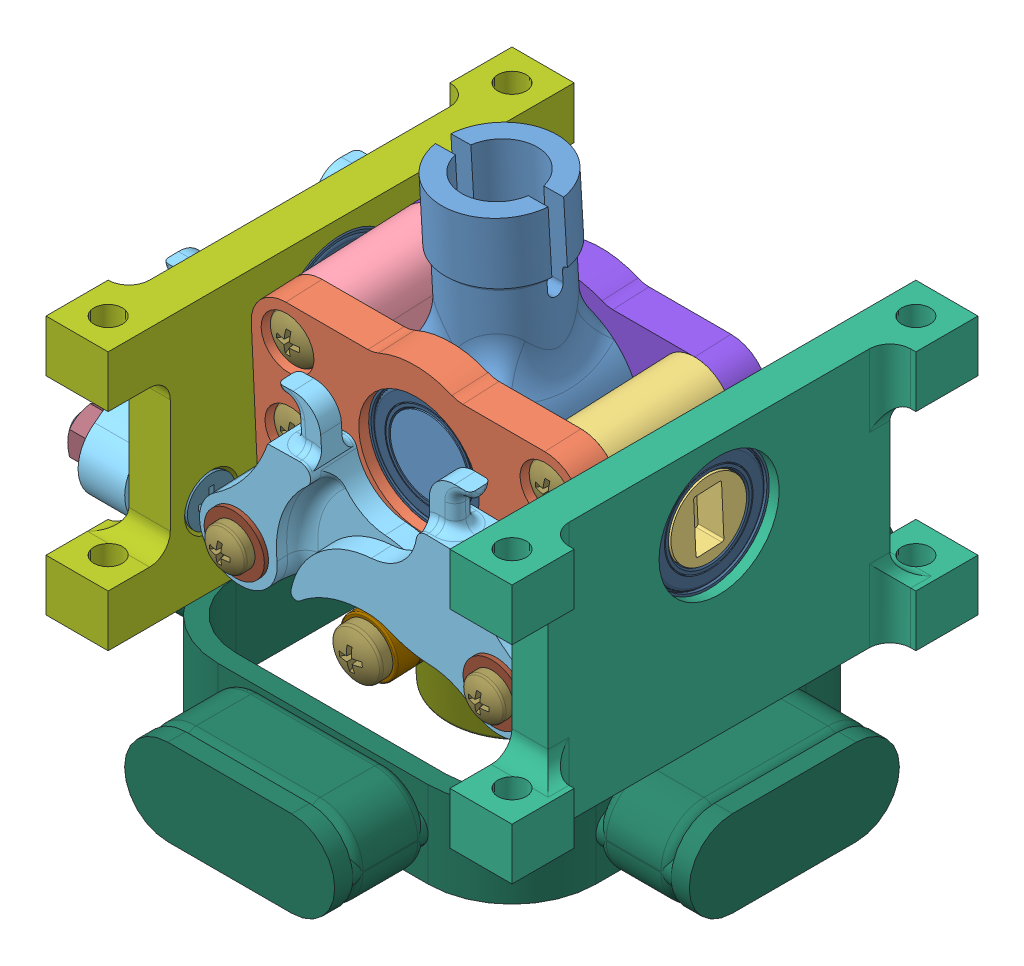
SolidWorks assembly gimbal, configuration Default. Lengths in mm.
Overall size (112.58 92.62 109.06).
47 component instances, 16 part files, 116 mates.
Components (placement in the parent):
- gimbal_lever_arm-1: gimbal_lever_arm [Default] at (47.4383 75.9682 -14.122) x (-0.999902 -0.01398 -0.000647) z (0 -0.046209 0.998932) size (30 86 35)
- gimbal_core_bearing_carrier_non_pot_side-1: gimbal_core_bearing_carrier_non_pot_side [Default] at (1 7.5205 9.7406) x (1 0 0) z (0 -0.046209 0.998932) size (64 44 7.5)
- gimbal_core_pot_side-1: gimbal_core_pot_side [Default] at (51 19.5077 10.2951) x (0 0.046209 -0.998932) z (1 0 0) size (22 30 20)
- gimbal_core_non_pot_side-1: gimbal_core_non_pot_side [Default] at (15 3.5756 -13.1836) x (0 -0.046209 0.998932) z (-1 0 0) size (23.38 47 23)
- gimbal_cam-1: gimbal_cam [Default] at (65.2863 3.5447 27.3757) x (-0.999775 0.021174 0.000979) z (0 0.046209 -0.998932) size (47.46 36.5 9)
- gimbal_cam-2: gimbal_cam [Default] at (0.7009 3.9697 18.3858) x (0.999801 0.01992 0.000921) z (0 -0.046209 0.998932) size (47.46 36.5 9)
- gimbal_frame_pot_side-1: gimbal_frame_pot_side [Default] at (66 0 45) x (0 0 -1) z (1 0 0) size (90 50 12)
- gimbal_frame_cam_side-1: gimbal_frame_cam_side [Default] at (0 0 -45) x (0 0 1) z (-1 0 0) size (90 50 12)
- gimbal_cam-3: gimbal_cam [Default] at (-18.3 4.8402 32.2821) x (0 0.021614 -0.999766) z (1 0 0) size (47.46 36.5 9)
- gimbal_cam-4: gimbal_cam [Default] at (-9.3 4.7894 -32.2106) x (0 0.028628 0.99959) z (-1 0 0) size (47.46 36.5 9)
- gimbal_core_bearing_carrier_pot_side-1: gimbal_core_bearing_carrier_pot_side [Default] at (65 18.027 -11.7969) x (-1 0 0) z (0 0.046209 -0.998932) size (64 34.5 7)
- 685 Bearing-1: 685 Bearing [По умолчанию] at (31.1601 10.3423 18.18) x (0 -0.046209 0.998932) z (-0.482505 -0.874958 -0.040474) size (5 11 11)
- 6802 Bearing-1: 6802 Bearing [Default] at (-2.5 35 0) x (1 0 0) z (0 -0.265463 0.964121) size (5 24 24)
- 6802 Bearing-2: 6802 Bearing [Default] at (68.5 35 0) x (1 0 0) z (0 -0.094888 0.995488) size (5 24 24)
- 6802 Bearing-3: 6802 Bearing [Default] at (33 34.3762 13.4856) x (0 0.046209 -0.998932) z (0.974697 -0.223291 -0.010329) size (5 24 24)
- 6802 Bearing-4: 6802 Bearing [Default] at (33 35.6238 -13.4856) x (0 -0.046209 0.998932) z (-0.998311 -0.058031 -0.002684) size (5 24 24)
- 685 Bearing-3: 685 Bearing [По умолчанию] at (-8.8 11.9085 -2.8011) x (-1 0 0) z (0 -0.658338 -0.752723) size (5 11 11)
- 685 Bearing-5: 685 Bearing [По умолчанию] at (-18.8 12.2864 -0.0857) x (1 0 0) z (0 -0.427815 0.903866) size (5 11 11)
- 685 Bearing-6: 685 Bearing [По умолчанию] at (33.1012 11.3912 23.2339) x (0 -0.046209 0.998932) z (-0.995039 -0.09938 -0.004597) size (5 11 11)
- MF105 Bearing-1: MF105 Bearing [Default] at (58 13.746 26.6463) x (-0.997509 0.070457 0.003259) z (0 0.046209 -0.998932) size (11.6 11.6 4)
- MF105 Bearing-2: MF105 Bearing [Default] at (58 14.051 20.0534) x (1 0 0) z (0 -0.046209 0.998932) size (11.6 11.6 4)
- MF105 Bearing-3: MF105 Bearing [Default] at (8 14.051 20.0534) x (1 0 0) z (0 -0.046209 0.998932) size (11.6 11.6 4)
- MF105 Bearing-4: MF105 Bearing [Default] at (8 13.746 26.6463) x (-0.996576 0.082596 0.003821) z (0 0.046209 -0.998932) size (11.6 11.6 4)
- MF105 Bearing-5: MF105 Bearing [Default] at (-10.5 15 25) x (0 0 1) z (-1 0 0) size (11.6 11.6 4)
- MF105 Bearing-6: MF105 Bearing [Default] at (-17.1 15 25) x (0 0.244393 -0.969676) z (1 0 0) size (11.6 11.6 4)
- MF105 Bearing-7: MF105 Bearing [Default] at (-17.1 15 -25) x (0 0 -1) z (1 0 0) size (11.6 11.6 4)
- MF105 Bearing-8: MF105 Bearing [Default] at (-10.5 15 -25) x (0 0 1) z (-1 0 0) size (11.6 11.6 4)
- pan cross head_am-1: pan cross head_am [B18.6.7M - M5 x 0.8 x 30 Type I Cross Recessed PHMS --30N] at (33.3499 8.5043 31.8096) x (0 0.046209 -0.998932) z (0.071714 -0.99636 -0.04609) size (33.67 9.5 9.5)
- pan cross head_am-2: pan cross head_am [B18.6.7M - M5 x 0.8 x 30 Type I Cross Recessed PHMS --30N] at (-22.5 10.0267 -1.1552) x (1 0 0) z (0 0.654485 0.756075) size (33.67 9.5 9.5)
- pan cross head_am-4: pan cross head_am [B18.6.7M - M4 x 0.7 x 20 Type I Cross Recessed PHMS --20N] at (8 13.5103 31.7409) x (0 0.046209 -0.998932) z (0.997483 -0.070827 -0.003276) size (23.07 8 8)
- pan cross head_am-5: pan cross head_am [B18.6.7M - M4 x 0.7 x 20 Type I Cross Recessed PHMS --20N] at (58 13.5103 31.7409) x (0 0.046209 -0.998932) z (0.997483 -0.070827 -0.003276) size (23.07 8 8)
- pan cross head_am-8: pan cross head_am [B18.6.7M - M5 x 0.8 x 35 Type I Cross Recessed PHMS --35N] at (58 42.1505 18.5502) x (0 0.046209 -0.998932) z (0.997483 -0.070827 -0.003276) size (38.67 9.5 9.5)
- pan cross head_am-9: pan cross head_am [B18.6.7M - M5 x 0.8 x 35 Type I Cross Recessed PHMS --35N] at (8 42.1505 18.5502) x (0 0.046209 -0.998932) z (0.997483 -0.070827 -0.003276) size (38.67 9.5 9.5)
- pan cross head_am-10: pan cross head_am [B18.6.7M - M5 x 0.8 x 35 Type I Cross Recessed PHMS --35N] at (8 26.1675 17.8109) x (0 0.046209 -0.998932) z (0.997483 -0.070827 -0.003276) size (38.67 9.5 9.5)
- pan cross head_am-11: pan cross head_am [B18.6.7M - M5 x 0.8 x 35 Type I Cross Recessed PHMS --35N] at (58 26.1675 17.8109) x (0 0.046209 -0.998932) z (0.997483 -0.070827 -0.003276) size (38.67 9.5 9.5)
- hex nut style 1_am-1: hex nut style 1_am [B18.2.4.1M - Hex nut, Style 1,  M5 x 0.8 --D-N] at (8 43.8787 -18.8098) x (0.866025 0.499466 0.023104) z (0 0.046209 -0.998932) size (8 9.24 4.7)
- hex nut style 1_am-2: hex nut style 1_am [B18.2.4.1M - Hex nut, Style 1,  M5 x 0.8 --D-N] at (8 27.8958 -19.5492) x (0.866025 0.499466 0.023104) z (0 0.046209 -0.998932) size (8 9.24 4.7)
- hex nut style 1_am-3: hex nut style 1_am [B18.2.4.1M - Hex nut, Style 1,  M5 x 0.8 --D-N] at (58 27.8958 -19.5492) x (0.866025 -0.499466 -0.023104) z (0 0.046209 -0.998932) size (8 9.24 4.7)
- hex nut style 1_am-4: hex nut style 1_am [B18.2.4.1M - Hex nut, Style 1,  M5 x 0.8 --D-N] at (58 43.8787 -18.8098) x (0.866025 -0.499466 -0.023104) z (0 0.046209 -0.998932) size (8 9.24 4.7)
- flat head screw_am-1: flat head screw_am [B18.6.7M - M5 x 0.8 x 25 Type I Cross Recessed FHMS --25N] at (-0.05 15 -25) x (-1 0 0) z (0 -0.000444 -1) size (25 9.3 9.3)
- flat head screw_am-2: flat head screw_am [B18.6.7M - M5 x 0.8 x 25 Type I Cross Recessed FHMS --25N] at (-0.05 15 25) x (-1 0 0) z (0 -0.006616 -0.999978) size (25 9.3 9.3)
- hex nut style 1_am-5: hex nut style 1_am [B18.2.4.1M - Hex nut, Style 1,  M5 x 0.8 --D-N] at (-23.8 15 25) x (0 0 1) z (-1 0 0) size (8 9.24 4.7)
- hex nut style 1_am-6: hex nut style 1_am [B18.2.4.1M - Hex nut, Style 1,  M5 x 0.8 --D-N] at (-23.8 15 -25) x (0 0 1) z (-1 0 0) size (8 9.24 4.7)
- hex nut style 1_am-9: hex nut style 1_am [B18.2.4.1M - Hex nut, Style 1,  M5 x 0.8 --D-N] at (58 14.5685 8.8654) x (0.866025 0.499466 0.023104) z (0 0.046209 -0.998932) size (8 9.24 4.7)
- hex nut style 1_am-10: hex nut style 1_am [B18.2.4.1M - Hex nut, Style 1,  M5 x 0.8 --D-N] at (8 14.5685 8.8654) x (0.866025 -0.499466 -0.023104) z (0 0.046209 -0.998932) size (8 9.24 4.7)
- gimbal_base-1: gimbal_base [Default] at (33 0 0) size (109.06 16.65 109.06)
- Magnetic Core-1: Magnetic Core [Default] at (33.6428 -10.8806 -2.1224) x (0.999902 0.01398 0.000647) z (0 -0.046209 0.998932) size (30 10 30)
Mates (geometry in assembly coordinates):
- Coincident1: coincident anti-aligned: plane of gimbal_core_bearing_carrier_non_pot_side-1 through (58 14.5131 10.0641) normal (0 0.046209 -0.998932); plane of gimbal_core_pot_side-1 through (58 42.4832 11.3579) normal (0 -0.046209 0.998932)
- Concentric2: concentric aligned: cylinder of gimbal_core_bearing_carrier_non_pot_side-1 through (58 42.4832 11.3579) axis (0 -0.046209 0.998932) radius 2.75; cylinder of gimbal_core_pot_side-1 through (58 43.4998 -10.6186) axis (0 -0.046209 0.998932) radius 2.75
- Concentric3: concentric aligned: cylinder of gimbal_core_bearing_carrier_non_pot_side-1 through (58 26.5002 10.6186) axis (0 -0.046209 0.998932) radius 2.75; cylinder of gimbal_core_pot_side-1 through (58 27.5168 -11.3579) axis (0 -0.046209 0.998932) radius 2.75
- Concentric4: concentric aligned: cylinder of gimbal_lever_arm-1 through (33 34.2607 15.9829) axis (0 0.046209 -0.998932) radius 7.5; cylinder of gimbal_core_bearing_carrier_non_pot_side-1 through (33 34.256 16.0828) axis (0 0.046209 -0.998932) radius 12.1
- Distance1: distance = 1 mm anti-aligned: plane of gimbal_core_bearing_carrier_non_pot_side-1 through (58 14.5131 10.0641) normal (0 0.046209 -0.998932); plane of gimbal_lever_arm-1 through (33 34.5379 9.9893) normal (0 -0.046209 0.998932)
- Coincident3: coincident anti-aligned: plane of gimbal_core_bearing_carrier_non_pot_side-1 through (58 14.5131 10.0641) normal (0 0.046209 -0.998932); plane of gimbal_core_non_pot_side-1 through (1 19.5077 10.2951) normal (0 -0.046209 0.998932)
- Concentric5: concentric anti-aligned: cylinder of gimbal_core_bearing_carrier_non_pot_side-1 through (8 42.4832 11.3579) axis (0 -0.046209 0.998932) radius 2.75; cylinder of gimbal_core_non_pot_side-1 through (8 42.9915 0.3697) axis (0 0.046209 -0.998932) radius 2.75
- Concentric6: concentric anti-aligned: cylinder of gimbal_core_bearing_carrier_non_pot_side-1 through (8 26.5002 10.6186) axis (0 -0.046209 0.998932) radius 2.75; cylinder of gimbal_core_non_pot_side-1 through (8 27.0085 -0.3697) axis (0 0.046209 -0.998932) radius 2.75
- Coincident4: coincident anti-aligned: plane of gimbal_core_non_pot_side-1 through (1 20.5243 -11.6814) normal (0 0.046209 -0.998932); plane of gimbal_core_bearing_carrier_non_pot_side-2 through (8 15.4069 -11.7093) normal (0 -0.03582 0.999358)
- Concentric7: concentric aligned: cylinder of gimbal_lever_arm-1 through (33 35.7393 -15.9829) axis (0 -0.046209 0.998932) radius 7.5; cylinder of gimbal_core_bearing_carrier_non_pot_side-2 through (33 35.5767 -16.0897) axis (0 -0.03582 0.999358) radius 12.1
- Concentric8: concentric aligned: cylinder of gimbal_core_non_pot_side-1 through (8 42.9915 0.3697) axis (0 0.046209 -0.998932) radius 2.75; cylinder of gimbal_core_bearing_carrier_non_pot_side-2 through (8 43.3889 -10.7064) axis (0 0.03582 -0.999358) radius 2.75
- Concentric9: concentric aligned: cylinder of gimbal_core_bearing_carrier_non_pot_side-1 through (58 14.5131 10.0641) axis (0 -0.046209 0.998932) radius 2.75; cylinder of gimbal_cam-1 through (58 13.8754 23.8493) axis (0 -0.046209 0.998932) radius 5.1
- Distance2: distance = 1.8 mm anti-aligned: plane of gimbal_cam-1 through (79.4969 44.8004 20.2745) normal (0 0.046209 -0.998932); plane of gimbal_core_bearing_carrier_non_pot_side-1 through (58 14.1896 17.0566) normal (0 -0.046209 0.998932)
- Distance3: distance = 1.8 mm anti-aligned: plane of gimbal_cam-2 through (-13.4583 44.8273 20.2758) normal (0 0.046209 -0.998932); plane of gimbal_core_bearing_carrier_non_pot_side-1 through (58 14.1896 17.0566) normal (0 -0.046209 0.998932)
- Concentric10: concentric anti-aligned: cylinder of gimbal_core_bearing_carrier_non_pot_side-1 through (8 14.5131 10.0641) axis (0 -0.046209 0.998932) radius 2.75; cylinder of gimbal_cam-2 through (8 13.9216 22.8504) axis (0 0.046209 -0.998932) radius 5.1
- Coincident7: coincident anti-aligned: plane of gimbal_frame_cam_side-1 through (-8 0 0) normal (0 -1 0)
- Coincident8: coincident aligned: plane of gimbal_frame_cam_side-1 through (0 0 -45) normal (1 0 0)
- Coincident9: coincident aligned: plane of gimbal_frame_cam_side-1 through (0 0 0) normal (0 0 1)
- Concentric11: concentric aligned: cylinder of gimbal_core_non_pot_side-1 through (-5 35 0) axis (1 0 0) radius 7.3; cylinder of gimbal_frame_cam_side-1 through (-5.1 35 0) axis (1 0 0) radius 12.1
- Distance4: distance = 1 mm anti-aligned: plane of gimbal_frame_cam_side-1 through (0 0 -45) normal (1 0 0); plane of gimbal_core_bearing_carrier_non_pot_side-1 through (1 42.1597 18.3504) normal (-1 0 0)
- Concentric12: concentric aligned: cylinder of gimbal_core_pot_side-1 through (71 35 0) axis (-1 0 0) radius 7.3; cylinder of gimbal_frame_pot_side-1 through (71.1 35 0) axis (-1 0 0) radius 12.15
- Coincident12: coincident anti-aligned: plane of gimbal_frame_pot_side-1 through (73 0 0) normal (0 -1 0)
- Distance5: distance = 1 mm anti-aligned: plane of gimbal_frame_pot_side-1 through (66 35 0) normal (-1 0 0); plane of gimbal_core_bearing_carrier_non_pot_side-1 through (65 42.1597 18.3504) normal (1 0 0)
- Distance6: distance = 1.3 mm anti-aligned: plane of gimbal_cam-3 through (-9.3 45.7178 46.5097) normal (1 0 0); plane of gimbal_frame_cam_side-1 through (-8 0 -45) normal (-1 0 0)
- Concentric13: concentric aligned: cylinder of gimbal_frame_cam_side-1 through (0 15 25) axis (-1 0 0) radius 2.75; cylinder of gimbal_cam-3 through (-14.3 15 25) axis (-1 0 0) radius 5.1
- Concentric14: concentric anti-aligned: cylinder of gimbal_frame_cam_side-1 through (0 15 -25) axis (-1 0 0) radius 2.75; cylinder of gimbal_cam-4 through (-13.3 15 -25) axis (1 0 0) radius 5.1
- Distance7: distance = 1.3 mm anti-aligned: plane of gimbal_cam-4 through (-9.3 45.5661 -46.7247) normal (1 0 0); plane of gimbal_frame_cam_side-1 through (-8 0 -45) normal (-1 0 0)
- Concentric16: concentric anti-aligned: cylinder of gimbal_lever_arm-1 through (33.3499 10.7685 -17.138) axis (0 -0.046209 0.998932) radius 2.75; cylinder of 685 Bearing-1 through (33.3499 9.1866 17.0585) axis (0 0.046209 -0.998932) radius 2.5
- Concentric18: concentric aligned: cylinder of gimbal_lever_arm-1 through (33.3499 10.7685 -17.138) axis (0 -0.046209 0.998932) radius 2.75; cylinder of pan cross head_am-1 through (33.3499 7.3306 57.1825) axis (0 -0.046209 0.998932) radius 2.5
- Concentric19: concentric anti-aligned: cylinder of gimbal_core_non_pot_side-1 through (-5 35 0) axis (1 0 0) radius 7.3; cylinder of 6802 Bearing-1 through (0 35 0) axis (-1 0 0) radius 7.5
- Coincident17: coincident anti-aligned: plane of gimbal_core_non_pot_side-1 through (0 35 0) normal (-1 0 0); plane of 6802 Bearing-1 through (0 35 0) normal (1 0 0)
- Concentric20: concentric aligned: cylinder of gimbal_core_pot_side-1 through (71 35 0) axis (-1 0 0) radius 7.3; cylinder of 6802 Bearing-2 through (71 35 0) axis (-1 0 0) radius 7.5
- Coincident18: coincident anti-aligned: plane of gimbal_core_pot_side-1 through (66 35 0) normal (1 0 0); plane of 6802 Bearing-2 through (66 35 0) normal (-1 0 0)
- Concentric21: concentric anti-aligned: cylinder of gimbal_lever_arm-1 through (33 34.2607 15.9829) axis (0 0.046209 -0.998932) radius 7.5; cylinder of 6802 Bearing-3 through (33 34.4917 10.9882) axis (0 -0.046209 0.998932) radius 7.5
- Coincident19: coincident anti-aligned: plane of gimbal_lever_arm-1 through (33 34.4917 10.9882) normal (0 -0.046209 0.998932); plane of 6802 Bearing-3 through (33 34.4917 10.9882) normal (0 0.046209 -0.998932)
- Concentric22: concentric anti-aligned: cylinder of gimbal_lever_arm-1 through (33 35.7393 -15.9829) axis (0 -0.046209 0.998932) radius 7.5; cylinder of 6802 Bearing-4 through (33 35.5083 -10.9882) axis (0 0.046209 -0.998932) radius 7.5
- Coincident20: coincident anti-aligned: plane of gimbal_lever_arm-1 through (33 35.5083 -10.9882) normal (0 0.046209 -0.998932); plane of 6802 Bearing-4 through (33 35.5083 -10.9882) normal (0 -0.046209 0.998932)
- LimitAngle2: limit planar angle = 0.013995 rad anti-aligned: plane of gimbal_lever_arm-1 through (32.4393 75.7585 -14.1317) normal (-0.999902 -0.01398 -0.000647)
- LimitAngle4: limit planar angle = 0.046225 rad anti-aligned: plane of gimbal_lever_arm-1 through (47.4383 75.2288 1.8609) normal (0 0.046209 -0.998932)
- Concentric23: concentric aligned: cylinder of gimbal_lever_arm-1 through (33 35.7393 -15.9829) axis (0 -0.046209 0.998932) radius 7.5; cylinder of gimbal_core_bearing_carrier_pot_side-1 through (33 35.744 -16.0828) axis (0 -0.046209 0.998932) radius 12.1
- Coincident23: coincident anti-aligned: plane of gimbal_core_non_pot_side-1 through (1 20.5243 -11.6814) normal (0 0.046209 -0.998932); plane of gimbal_core_bearing_carrier_pot_side-1 through (58 27.5168 -11.3579) normal (0 -0.046209 0.998932)
- Concentric24: concentric anti-aligned: cylinder of gimbal_core_non_pot_side-1 through (8 42.9915 0.3697) axis (0 0.046209 -0.998932) radius 2.75; cylinder of gimbal_core_bearing_carrier_pot_side-1 through (8 43.8232 -17.6111) axis (0 -0.046209 0.998932) radius 2.75
- Concentric25: concentric anti-aligned: cylinder of gimbal_core_non_pot_side-1 through (15 10.0267 -1.1552) axis (-1 0 0) radius 2.75; cylinder of 685 Bearing-3 through (-7.7331 10.0267 -1.1552) axis (1 0 0) radius 2.5
- Concentric26: concentric aligned: cylinder of gimbal_core_non_pot_side-1 through (15 10.0267 -1.1552) axis (-1 0 0) radius 2.75; cylinder of pan cross head_am-2 through (-47.9 10.0267 -1.1552) axis (-1 0 0) radius 2.5
- PathMate2: path: point of 685 Bearing-3; curve of gimbal_cam-4; curve of gimbal_cam-4
- Concentric27: concentric aligned: cylinder of gimbal_core_non_pot_side-1 through (15 10.0267 -1.1552) axis (-1 0 0) radius 2.75; cylinder of 685 Bearing-5 through (-19.8669 10.0267 -1.1552) axis (-1 0 0) radius 2.5
- PathMate3: path: point of 685 Bearing-5; curve of gimbal_cam-3; curve of gimbal_cam-3
- Coincident27: coincident anti-aligned: plane of pan cross head_am-2 through (-18.8 11.9169 -2.7914) normal (1 0 0); plane of 685 Bearing-5 through (-18.8 12.2864 -0.0857) normal (-1 0 0)
- PathMate4: path: unknown of 685 Bearing-1; edge_curve of ?
- Concentric28: concentric anti-aligned: cylinder of gimbal_lever_arm-1 through (33.3499 10.7685 -17.138) axis (0 -0.046209 0.998932) radius 2.75; cylinder of 685 Bearing-6 through (33.3499 8.9556 22.0532) axis (0 0.046209 -0.998932) radius 2.5
- PathMate5: path: point of 685 Bearing-6; curve of gimbal_cam-1; curve of gimbal_cam-1
- Coincident28: coincident anti-aligned: plane of pan cross head_am-1 through (35.8434 8.8543 28.1219) normal (0 0.046209 -0.998932); plane of 685 Bearing-6 through (33.1012 11.1602 28.2285) normal (0 -0.046209 0.998932)
- Concentric29: concentric anti-aligned: cylinder of gimbal_cam-1 through (58 13.8754 23.8493) axis (0 -0.046209 0.998932) radius 5.1; cylinder of MF105 Bearing-1 through (58 13.746 26.6463) axis (0 0.046209 -0.998932) radius 5
- Coincident29: coincident anti-aligned: plane of gimbal_cam-1 through (79.4969 44.3845 29.2649) normal (0 -0.046209 0.998932); plane of MF105 Bearing-1 through (58.3527 18.6728 28.0755) normal (0 0.046209 -0.998932)
- Coincident30: coincident anti-aligned: plane of gimbal_cam-1 through (79.4969 44.8004 20.2745) normal (0 0.046209 -0.998932); plane of MF105 Bearing-2 through (58 19.1011 19.0857) normal (0 -0.046209 0.998932)
- Concentric30: concentric aligned: cylinder of gimbal_cam-1 through (58 13.8754 23.8493) axis (0 -0.046209 0.998932) radius 5.1; cylinder of MF105 Bearing-2 through (58 14.051 20.0534) axis (0 -0.046209 0.998932) radius 5
- Coincident31: coincident anti-aligned: plane of gimbal_cam-2 through (-13.4583 44.8273 20.2758) normal (0 0.046209 -0.998932); plane of MF105 Bearing-3 through (8 19.1011 19.0857) normal (0 -0.046209 0.998932)
- Concentric31: concentric anti-aligned: cylinder of gimbal_cam-2 through (8 13.9216 22.8504) axis (0 0.046209 -0.998932) radius 5.1; cylinder of MF105 Bearing-3 through (8 14.051 20.0534) axis (0 -0.046209 0.998932) radius 5
- Coincident32: coincident anti-aligned: plane of gimbal_cam-2 through (-13.4583 44.4114 29.2662) normal (0 -0.046209 0.998932); plane of MF105 Bearing-4 through (8.4134 18.6681 28.0753) normal (0 0.046209 -0.998932)
- Concentric32: concentric aligned: cylinder of gimbal_cam-2 through (8 13.9216 22.8504) axis (0 0.046209 -0.998932) radius 5.1; cylinder of MF105 Bearing-4 through (8 13.746 26.6463) axis (0 0.046209 -0.998932) radius 5
- Concentric33: concentric anti-aligned: cylinder of gimbal_cam-3 through (-14.3 15 25) axis (-1 0 0) radius 5.1; cylinder of MF105 Bearing-6 through (-17.1 15 25) axis (1 0 0) radius 5
- Coincident33: coincident anti-aligned: plane of gimbal_cam-3 through (-18.3 45.7178 46.5097) normal (-1 0 0); plane of MF105 Bearing-6 through (-18.3 19.8484 26.222) normal (1 0 0)
- Coincident34: coincident anti-aligned: plane of gimbal_cam-3 through (-9.3 45.7178 46.5097) normal (1 0 0); plane of MF105 Bearing-5 through (-9.3 20 25) normal (-1 0 0)
- Concentric34: concentric aligned: cylinder of gimbal_cam-3 through (-14.3 15 25) axis (-1 0 0) radius 5.1; cylinder of MF105 Bearing-5 through (-10.5 15 25) axis (-1 0 0) radius 5
- Coincident35: coincident anti-aligned: plane of gimbal_cam-4 through (-18.3 45.5661 -46.7247) normal (-1 0 0); plane of MF105 Bearing-7 through (-18.3 20 -25) normal (1 0 0)
- Concentric35: concentric aligned: cylinder of gimbal_cam-4 through (-13.3 15 -25) axis (1 0 0) radius 5.1; cylinder of MF105 Bearing-7 through (-17.1 15 -25) axis (1 0 0) radius 5
- Coincident36: coincident anti-aligned: plane of gimbal_cam-4 through (-9.3 45.5661 -46.7247) normal (1 0 0); plane of MF105 Bearing-8 through (-9.3 20 -25) normal (-1 0 0)
- Concentric36: concentric anti-aligned: cylinder of gimbal_cam-4 through (-13.3 15 -25) axis (1 0 0) radius 5.1; cylinder of MF105 Bearing-8 through (-10.5 15 -25) axis (-1 0 0) radius 5
- Concentric371: concentric anti-aligned: cylinder of MF105 Bearing-4 through (8 13.746 26.6463) axis (0 0.046209 -0.998932) radius 2.5; cylinder of pan cross head_am-3 through (8 19.2123 59.9703) axis (0 0.070903 0.997483) radius 2.5
- Coincident371: coincident anti-aligned: plane of MF105 Bearing-4 through (8.2067 16.1424 28.7593) normal (0 -0.046209 0.998932); plane of pan cross head_am-3 through (10.4836 17.4346 30.9233) normal (0 -0.070903 -0.997483)
- Concentric38: concentric anti-aligned: cone of MF105 Bearing-4 through (8 13.6536 28.6442) axis (0 0.046209 -0.998932); cylinder of pan cross head_am-4 through (8 12.3366 57.1138) axis (0 -0.046209 0.998932) radius 4
- Coincident38: coincident anti-aligned: plane of MF105 Bearing-4 through (8.2067 16.1424 28.7593) normal (0 -0.046209 0.998932); plane of pan cross head_am-4 through (8.1418 15.6464 28.7364) normal (0 0.046209 -0.998932)
- Concentric39: concentric anti-aligned: cone of MF105 Bearing-1 through (58 13.6536 28.6442) axis (0 0.046209 -0.998932); cylinder of pan cross head_am-5 through (58 12.3366 57.1138) axis (0 -0.046209 0.998932) radius 4
- Coincident39: coincident anti-aligned: plane of MF105 Bearing-1 through (58.1763 16.1447 28.7594) normal (0 -0.046209 0.998932); plane of pan cross head_am-5 through (58.1418 15.6464 28.7364) normal (0 0.046209 -0.998932)
- Concentric40: concentric anti-aligned: cone of MF105 Bearing-6 through (-19.1 15 25) axis (1 0 0); cylinder of pan cross head_am-6 through (-47.6 15 25) axis (-1 0 0) radius 4
- Coincident40: coincident anti-aligned: plane of MF105 Bearing-6 through (-19.1 17.4242 25.611) normal (-1 0 0); plane of pan cross head_am-6 through (-19.1 17 25) normal (1 0 0)
- Concentric41: concentric anti-aligned: cone of MF105 Bearing-7 through (-19.1 15 -25) axis (1 0 0); cylinder of pan cross head_am-7 through (-47.6 15 -25) axis (-1 0 0) radius 4
- Coincident41: coincident anti-aligned: plane of MF105 Bearing-7 through (-19.1 17.5 -25) normal (-1 0 0); plane of pan cross head_am-7 through (-19.1 17 -25) normal (1 0 0)
- Concentric42: concentric aligned: cylinder of gimbal_core_bearing_carrier_non_pot_side-1 through (58 42.4832 11.3579) axis (0 -0.046209 0.998932) radius 2.75; cylinder of pan cross head_am-8 through (58 40.9768 43.9231) axis (0 -0.046209 0.998932) radius 4.75
- Coincident42: coincident anti-aligned: plane of gimbal_core_bearing_carrier_non_pot_side-1 through (58 42.3214 14.8542) normal (0 -0.046209 0.998932); plane of pan cross head_am-8 through (58.1773 44.8125 14.9694) normal (0 0.046209 -0.998932)
- Concentric43: concentric aligned: cylinder of gimbal_core_bearing_carrier_non_pot_side-1 through (8 42.4832 11.3579) axis (0 -0.046209 0.998932) radius 2.75; cylinder of pan cross head_am-9 through (8 40.9768 43.9231) axis (0 -0.046209 0.998932) radius 4.75
- Coincident43: coincident anti-aligned: plane of gimbal_core_bearing_carrier_non_pot_side-1 through (8 42.3214 14.8542) normal (0 -0.046209 0.998932); plane of pan cross head_am-9 through (8.1773 44.8125 14.9694) normal (0 0.046209 -0.998932)
- Concentric44: concentric aligned: cylinder of gimbal_core_bearing_carrier_non_pot_side-1 through (8 26.5002 10.6186) axis (0 -0.046209 0.998932) radius 2.75; cylinder of pan cross head_am-10 through (8 24.9938 43.1838) axis (0 -0.046209 0.998932) radius 4.75
- Coincident44: coincident anti-aligned: plane of gimbal_core_bearing_carrier_non_pot_side-1 through (8 26.3385 14.1148) normal (0 -0.046209 0.998932); plane of pan cross head_am-10 through (8.1773 28.8296 14.2301) normal (0 0.046209 -0.998932)
- Concentric45: concentric aligned: cylinder of gimbal_core_bearing_carrier_non_pot_side-1 through (58 26.3385 14.1148) axis (0 -0.046209 0.998932) radius 5.1; cylinder of pan cross head_am-11 through (58 24.9938 43.1838) axis (0 -0.046209 0.998932) radius 4.75
- Coincident45: coincident anti-aligned: plane of gimbal_core_bearing_carrier_non_pot_side-1 through (58 26.3385 14.1148) normal (0 -0.046209 0.998932); plane of pan cross head_am-11 through (58.1773 28.8296 14.2301) normal (0 0.046209 -0.998932)
- Concentric46: concentric anti-aligned: cylinder of gimbal_core_bearing_carrier_pot_side-1 through (8 43.8232 -17.6111) axis (0 -0.046209 0.998932) radius 2.75; cylinder of hex nut style 1_am-1 through (8 42.7217 6.2009) axis (0 0.046209 -0.998932) radius 2.5
- Coincident46: coincident anti-aligned: plane of gimbal_core_bearing_carrier_pot_side-1 through (1 18.1887 -15.2932) normal (0 0.046209 -0.998932); plane of hex nut style 1_am-1 through (10.3094 39.6658 -14.2997) normal (0 -0.046209 0.998932)
- Concentric47: concentric anti-aligned: cylinder of gimbal_core_bearing_carrier_pot_side-1 through (8 27.8403 -18.3504) axis (0 -0.046209 0.998932) radius 2.75; cylinder of hex nut style 1_am-2 through (8 26.7388 5.4616) axis (0 0.046209 -0.998932) radius 2.5
- Coincident47: coincident anti-aligned: plane of gimbal_core_bearing_carrier_pot_side-1 through (1 18.1887 -15.2932) normal (0 0.046209 -0.998932); plane of hex nut style 1_am-2 through (10.3094 23.6828 -15.039) normal (0 -0.046209 0.998932)
- Concentric48: concentric anti-aligned: cylinder of gimbal_core_bearing_carrier_pot_side-1 through (58 27.8403 -18.3504) axis (0 -0.046209 0.998932) radius 2.75; cylinder of hex nut style 1_am-3 through (58 26.7388 5.4616) axis (0 0.046209 -0.998932) radius 2.5
- Coincident48: coincident anti-aligned: plane of gimbal_core_bearing_carrier_pot_side-1 through (65 18.1887 -15.2932) normal (0 0.046209 -0.998932); plane of hex nut style 1_am-3 through (55.6906 23.6828 -15.039) normal (0 -0.046209 0.998932)
- Concentric49: concentric anti-aligned: cylinder of gimbal_core_bearing_carrier_pot_side-1 through (58 43.8232 -17.6111) axis (0 -0.046209 0.998932) radius 2.75; cylinder of hex nut style 1_am-4 through (58 42.7217 6.2009) axis (0 0.046209 -0.998932) radius 2.5
- Coincident49: coincident anti-aligned: plane of gimbal_core_bearing_carrier_pot_side-1 through (65 18.1887 -15.2932) normal (0 0.046209 -0.998932); plane of hex nut style 1_am-4 through (55.6906 39.6658 -14.2997) normal (0 -0.046209 0.998932)
- Parallel31: parallel anti-aligned: plane of gimbal_core_bearing_carrier_pot_side-1 through (10.4537 47.9069 -13.9185) normal (0 -0.998932 -0.046209); plane of hex nut style 1_am-1 through (5.6906 47.6572 -13.93) normal (0 0.998932 0.046209)
- Parallel41: parallel anti-aligned: plane of gimbal_core_bearing_carrier_pot_side-1 through (10.4537 31.924 -14.6578) normal (0 -0.998932 -0.046209); plane of hex nut style 1_am-2 through (5.6906 31.6743 -14.6693) normal (0 0.998932 0.046209)
- Parallel51: parallel anti-aligned: plane of gimbal_core_bearing_carrier_pot_side-1 through (55.5463 31.924 -14.6578) normal (0 -0.998932 -0.046209); plane of hex nut style 1_am-3 through (55.6906 31.6743 -14.6693) normal (0 0.998932 0.046209)
- Parallel61: parallel anti-aligned: plane of gimbal_core_bearing_carrier_pot_side-1 through (55.5463 47.9069 -13.9185) normal (0 -0.998932 -0.046209); plane of hex nut style 1_am-4 through (55.6906 47.6572 -13.93) normal (0 0.998932 0.046209)
- Coincident372: coincident aligned: cone of gimbal_frame_cam_side-1 through (-2.5 15 -25) axis (-1 0 0); cone of flat head screw_am-1 through (-0.6 15 -25) axis (-1 0 0)
- Coincident373: coincident aligned: cone of gimbal_frame_cam_side-1 through (0 15 25) axis (-1 0 0); cone of flat head screw_am-2 through (-0.6 15 25) axis (-1 0 0)
- Concentric372: concentric anti-aligned: cone of MF105 Bearing-6 through (-19.1 15 25) axis (1 0 0); cylinder of hex nut style 1_am-5 through (1.2375 15 25) axis (-1 0 0) radius 2.5
- Coincident374: coincident anti-aligned: plane of MF105 Bearing-6 through (-19.1 17.4242 25.611) normal (-1 0 0); plane of hex nut style 1_am-5 through (-19.1 19.6188 25) normal (1 0 0)
- Concentric373: concentric anti-aligned: cone of MF105 Bearing-7 through (-19.1 15 -25) axis (1 0 0); cylinder of hex nut style 1_am-6 through (1.2375 15 -25) axis (-1 0 0) radius 2.5
- Coincident375: coincident anti-aligned: plane of MF105 Bearing-7 through (-19.1 17.5 -25) normal (-1 0 0); plane of hex nut style 1_am-6 through (-19.1 19.6188 -25) normal (1 0 0)
- Concentric376: concentric anti-aligned: cylinder of gimbal_core_bearing_carrier_non_pot_side-1 through (58 14.5131 10.0641) axis (0 -0.046209 0.998932) radius 2.75; cylinder of hex nut style 1_am-9 through (58 13.4116 33.8761) axis (0 0.046209 -0.998932) radius 2.5
- Coincident378: coincident anti-aligned: plane of gimbal_core_bearing_carrier_non_pot_side-1 through (1 7.3588 13.2369) normal (0 0.046209 -0.998932); plane of hex nut style 1_am-9 through (60.3094 10.3556 13.3755) normal (0 -0.046209 0.998932)
- Concentric377: concentric anti-aligned: cylinder of gimbal_core_bearing_carrier_non_pot_side-1 through (8 14.5131 10.0641) axis (0 -0.046209 0.998932) radius 2.75; cylinder of hex nut style 1_am-10 through (8 13.4116 33.8761) axis (0 0.046209 -0.998932) radius 2.5
- Coincident379: coincident anti-aligned: plane of gimbal_core_bearing_carrier_non_pot_side-1 through (65 7.3588 13.2369) normal (0 0.046209 -0.998932); plane of hex nut style 1_am-10 through (5.6906 10.3556 13.3755) normal (0 -0.046209 0.998932)
- Parallel62: parallel anti-aligned: plane of gimbal_core_bearing_carrier_non_pot_side-1 through (60.4537 10.1059 13.3639) normal (0 0.998932 0.046209); plane of hex nut style 1_am-9 through (60.3094 10.3556 13.3755) normal (0 -0.998932 -0.046209)
- Parallel63: parallel anti-aligned: plane of gimbal_core_bearing_carrier_non_pot_side-1 through (3.0925 14.3513 13.5603) normal (0.866025 0.499466 0.023104); plane of hex nut style 1_am-10 through (5.6906 10.3556 13.3755) normal (-0.866025 -0.499466 -0.023104)
- Tangent1: tangent aligned: cylinder of gimbal_lever_arm-1 through (32.6072 63.0331 1.2968) axis (-0.013995 0.998834 0.046204) radius 11; face of ?
- Parallel64: parallel aligned: cylinder of gimbal_lever_arm-1 through (32.6072 63.0331 1.2968) axis (-0.013995 0.998834 0.046204) radius 11; cylinder of Cobra Grip-1 through (10.771 77.6987 -10.051) axis (-0.02783 0.999408 0.020228) radius 15.5745
- Coincident382: coincident: unknown of gimbal_frame_cam_side-1
- Coincident383: coincident aligned: plane of gimbal_lever_arm-1 through (33.6428 -10.8806 -2.1224) normal (0.013995 -0.998834 -0.046204); plane of Magnetic Core-1 through (33.6428 -10.8806 -2.1224) normal (0.013995 -0.998834 -0.046204)
- Concentric378: concentric anti-aligned: cylinder of gimbal_lever_arm-1 through (33.6428 -10.8806 -2.1224) axis (-0.013995 0.998834 0.046204) radius 5.0399; cylinder of Magnetic Core-1 through (33.5029 -0.8923 -1.6603) axis (0.013995 -0.998834 -0.046204) radius 15
- Parallel65: parallel aligned: plane of gimbal_lever_arm-1 through (47.4383 75.9682 -14.122) normal (0 -0.046209 0.998932); plane of Magnetic Core-1 through (33.6428 -10.8806 -2.1224) normal (0 -0.046209 0.998932)
